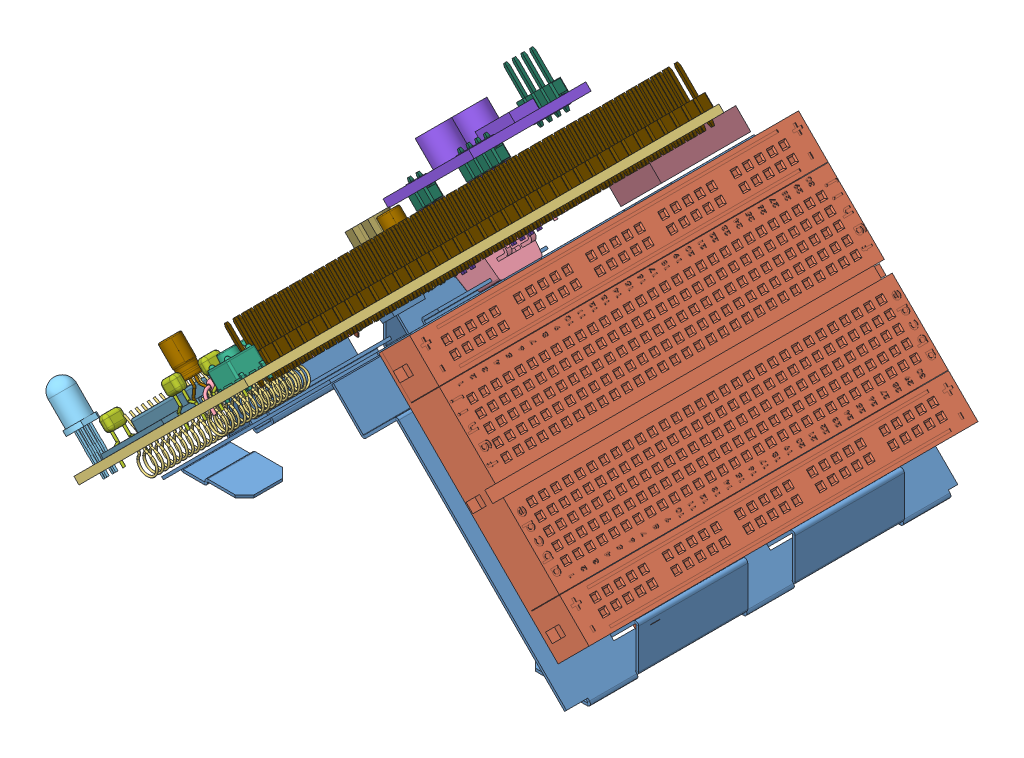
SolidWorks assembly board holder, configuration Default. Lengths in mm.
Overall size (106.21 104.29 116.2).
93 component instances, 22 part files, 18 mates.
Components (placement in the parent):
- board holder-1: board holder [Default] at (0.5717 42.6452 0.4358) x (0 0 -1) z (-0.707107 -0.707107 0) size (82.5 68.22 68.22)
- Breadboard 400-1: Breadboard 400 [Default] at (20.1582 24.8342 -10.9913) x (0 0 1) z (-0.707107 0.707107 0) size (83.85 9.2 55.35)
- MSE_duinoR5_1a-1: MSE_duinoR5_1a [Default] at (-32.0399 20.1527 23.2606) x (-0.00206 -0.00206 -0.999996) z (0.707104 0.707104 -0.002913) size (116.05 27.86 50.4)
  - flexypin-1: flexypin [Default] at (-20.41 0.2848 13.3424) x (-0.010953 -0.001001 0.99994) z (-0.000011 0.999999 0.001001) size (4.48 0.4 10.4)
  - flexypin-2: flexypin [Default] at (-19.14 0.2848 13.3424) x (-0.010953 -0.001001 0.99994) z (-0.000011 0.999999 0.001001) size (4.48 0.4 10.4)
  - flexypin-3: flexypin [Default] at (-17.87 0.2848 13.3424) x (-0.010953 -0.001001 0.99994) z (-0.000011 0.999999 0.001001) size (4.48 0.4 10.4)
  - flexypin-4: flexypin [Default] at (-16.6 0.2848 13.3424) x (-0.010953 -0.001001 0.99994) z (-0.000011 0.999999 0.001001) size (4.48 0.4 10.4)
  - flexypin-5: flexypin [Default] at (-15.33 0.2848 13.3424) x (-0.010953 -0.001001 0.99994) z (-0.000011 0.999999 0.001001) size (4.48 0.4 10.4)
  - flexypin-6: flexypin [Default] at (-14.06 0.2848 13.3424) x (-0.010953 -0.001001 0.99994) z (-0.000011 0.999999 0.001001) size (4.48 0.4 10.4)
  - flexypin-7: flexypin [Default] at (-12.79 0.2848 13.3424) x (-0.010953 -0.001001 0.99994) z (-0.000011 0.999999 0.001001) size (4.48 0.4 10.4)
  - flexypin-8: flexypin [Default] at (-11.52 0.2848 13.3424) x (-0.010953 -0.001001 0.99994) z (-0.000011 0.999999 0.001001) size (4.48 0.4 10.4)
  - flexypin-9: flexypin [Default] at (-10.25 0.2848 13.3424) x (-0.010953 -0.001001 0.99994) z (-0.000011 0.999999 0.001001) size (4.48 0.4 10.4)
  - flexypin-10: flexypin [Default] at (-8.98 0.2848 13.3424) x (-0.010953 -0.001001 0.99994) z (-0.000011 0.999999 0.001001) size (4.48 0.4 10.4)
  - flexypin-11: flexypin [Default] at (-7.71 0.2848 13.3424) x (-0.010953 -0.001001 0.99994) z (-0.000011 0.999999 0.001001) size (4.48 0.4 10.4)
  - flexypin-12: flexypin [Default] at (-6.44 0.2848 13.3424) x (-0.010953 -0.001001 0.99994) z (-0.000011 0.999999 0.001001) size (4.48 0.4 10.4)
  - flexypin-13: flexypin [Default] at (-5.17 0.2848 13.3424) x (-0.010953 -0.001001 0.99994) z (-0.000011 0.999999 0.001001) size (4.48 0.4 10.4)
  - flexypin-14: flexypin [Default] at (-3.9 0.2848 13.3424) x (-0.010953 -0.001001 0.99994) z (-0.000011 0.999999 0.001001) size (4.48 0.4 10.4)
  - flexypin-15: flexypin [Default] at (-0.8568 0.1483 9.8155) x (-0.999939 -0.001001 -0.010978) z (-0.001001 0.999999 -0.000011) size (4.48 0.4 10.4)
  - flexypin-16: flexypin [Default] at (-20.41 0.1483 -7.5876) x (-0.003303 -0.001001 0.999994) z (-0.000003 0.999999 0.001001) size (4.48 0.4 10.4)
  - flexypin-17: flexypin [Default] at (-0.8568 0.1483 8.5455) x (-0.999939 -0.001001 -0.010978) z (-0.001001 0.999999 -0.000011) size (4.48 0.4 10.4)
  - flexypin-18: flexypin [Default] at (-0.8568 0.1483 7.2755) x (-0.999939 -0.001001 -0.010978) z (-0.001001 0.999999 -0.000011) size (4.48 0.4 10.4)
  - flexypin-19: flexypin [Default] at (-0.8568 0.1483 6.0055) x (-0.999939 -0.001001 -0.010978) z (-0.001001 0.999999 -0.000011) size (4.48 0.4 10.4)
  - flexypin-20: flexypin [Default] at (-0.8568 0.1483 4.7355) x (-0.999939 -0.001001 -0.010978) z (-0.001001 0.999999 -0.000011) size (4.48 0.4 10.4)
  - flexypin-21: flexypin [Default] at (-0.8568 0.1483 3.4655) x (-0.999939 -0.001001 -0.010978) z (-0.001001 0.999999 -0.000011) size (4.48 0.4 10.4)
  - flexypin-22: flexypin [Default] at (-0.8568 0.1483 2.1955) x (-0.999939 -0.001001 -0.010978) z (-0.001001 0.999999 -0.000011) size (4.48 0.4 10.4)
  - flexypin-23: flexypin [Default] at (-0.8568 0.1483 0.9255) x (-0.999939 -0.001001 -0.010978) z (-0.001001 0.999999 -0.000011) size (4.48 0.4 10.4)
  - flexypin-24: flexypin [Default] at (-0.8568 0.1483 -0.3445) x (-0.999939 -0.001001 -0.010978) z (-0.001001 0.999999 -0.000011) size (4.48 0.4 10.4)
  - flexypin-25: flexypin [Default] at (-0.8568 0.1483 -1.6145) x (-0.999939 -0.001001 -0.010978) z (-0.001001 0.999999 -0.000011) size (4.48 0.4 10.4)
  - flexypin-26: flexypin [Default] at (-0.8568 0.1483 -2.8845) x (-0.999939 -0.001001 -0.010978) z (-0.001001 0.999999 -0.000011) size (4.48 0.4 10.4)
  - flexypin-27: flexypin [Default] at (-0.8568 0.1483 -4.1545) x (-0.999939 -0.001001 -0.010978) z (-0.001001 0.999999 -0.000011) size (4.48 0.4 10.4)
  - flexypin-28: flexypin [Default] at (-19.14 0.1483 -7.5876) x (-0.003303 -0.001001 0.999994) z (-0.000003 0.999999 0.001001) size (4.48 0.4 10.4)
  - flexypin-29: flexypin [Default] at (-17.87 0.1483 -7.5876) x (-0.003303 -0.001001 0.999994) z (-0.000003 0.999999 0.001001) size (4.48 0.4 10.4)
  - flexypin-30: flexypin [Default] at (-16.6 0.1483 -7.5876) x (-0.003303 -0.001001 0.999994) z (-0.000003 0.999999 0.001001) size (4.48 0.4 10.4)
  - flexypin-31: flexypin [Default] at (-15.33 0.1483 -7.5876) x (-0.003303 -0.001001 0.999994) z (-0.000003 0.999999 0.001001) size (4.48 0.4 10.4)
  - flexypin-32: flexypin [Default] at (-14.06 0.1483 -7.5876) x (-0.003303 -0.001001 0.999994) z (-0.000003 0.999999 0.001001) size (4.48 0.4 10.4)
  - flexypin-33: flexypin [Default] at (-12.79 0.1483 -7.5876) x (-0.003303 -0.001001 0.999994) z (-0.000003 0.999999 0.001001) size (4.48 0.4 10.4)
  - flexypin-34: flexypin [Default] at (-11.52 0.1483 -7.5876) x (-0.003303 -0.001001 0.999994) z (-0.000003 0.999999 0.001001) size (4.48 0.4 10.4)
  - flexypin-35: flexypin [Default] at (-10.25 0.1483 -7.5876) x (-0.003303 -0.001001 0.999994) z (-0.000003 0.999999 0.001001) size (4.48 0.4 10.4)
  - flexypin-36: flexypin [Default] at (-8.98 0.1483 -7.5876) x (-0.003303 -0.001001 0.999994) z (-0.000003 0.999999 0.001001) size (4.48 0.4 10.4)
  - flexypin-37: flexypin [Default] at (-7.71 0.1483 -7.5876) x (-0.003303 -0.001001 0.999994) z (-0.000003 0.999999 0.001001) size (4.48 0.4 10.4)
  - flexypin-38: flexypin [Default] at (-6.44 0.1483 -7.5876) x (-0.003303 -0.001001 0.999994) z (-0.000003 0.999999 0.001001) size (4.48 0.4 10.4)
  - flexypin-39: flexypin [Default] at (-5.17 0.1483 -7.5876) x (-0.003303 -0.001001 0.999994) z (-0.000003 0.999999 0.001001) size (4.48 0.4 10.4)
  - flexypin-40: flexypin [Default] at (-3.9 0.1483 -7.5876) x (-0.003303 -0.001001 0.999994) z (-0.000003 0.999999 0.001001) size (4.48 0.4 10.4)
  - 4k7 Resistor-2: 4k7 Resistor [Default] at (53.3526 1.6846 -2.2179) x (1 -0.000227 0) z (0 0 1) size (10.63 5.13 2.14)
  - 4k7 Resistor-3: 4k7 Resistor [Default] at (53.4006 1.1919 4.1961) x (1 -0.000227 0) z (0 0 1) size (10.63 5.13 2.14)
  - 4k7 Resistor-4: 4k7 Resistor [Default] at (53.3476 1.5334 20.6721) x (1 -0.000227 0) z (0 0 1) size (10.63 5.13 2.14)
  - 4k7 Resistor-5: 4k7 Resistor [Default] at (40.5664 1.561 -1.0614) x (1 -0.000286 0) z (0 0 1) size (10.63 5.13 2.14)
  - 4k7 Resistor-6: 4k7 Resistor [Default] at (17.8933 1.5357 -12.7339) x (-1 -0.000286 0) z (0 0 -1) size (10.63 5.13 2.14)
  - 4k7 Resistor-8: 4k7 Resistor [Default] at (53.4026 1.5613 0.9311) x (1 -0.000227 0) z (0 0 1) size (10.63 5.13 2.14)
  - APA-106-F8-1: APA-106-F8 [Default] at (-24.7776 1.0639 -10.8804) x (1 0 0) z (0 1 0) size (5.8 5.34 16.88)
  - B3F-10XX-1: B3F-10XX [Default] at (-24.9981 -0.2 31.2137) x (0.011028 0 0.999939) z (0 1 0) size (6.85 6 7)
  - B3F-10XX-2: B3F-10XX [Default] at (8.2644 -0.2 -9.7242) x (-0.011162 0 -0.999938) z (0 1 0) size (6.85 6 7)
  - C050024X044_C050024X044-1: C050024X044_C050024X044 [Default] at (13.928 -2.6 11.4866) x (0 0 -1) z (0 1 0) size (5.59 2.2 8.4)
  - C050024X044_C050024X044-2: C050024X044_C050024X044 [Default] at (23.427 -2.6 11.5366) x (0 0 -1) z (0 1 0) size (5.59 2.2 8.4)
  - C050024X044_C050024X044-3: C050024X044_C050024X044 [Default] at (-26.23 -2.6 16.8966) x (0 0 -1) z (0 1 0) size (5.59 2.2 8.4)
  - C050024X044_C050024X044-4: C050024X044_C050024X044 [Default] at (62.1347 -2.5253 11.5231) x (0 0 -1) z (0 1 0) size (5.59 2.2 8.4)
  - dual motor controller-1: dual motor controller [Default] at (49.5705 11.1526 10.8742) x (0.010236 0 0.999948) z (-0.999948 0 0.010236) size (25.07 7.1 24.93)
  - Electrolitic Capacitor Radial 4x7-1: Electrolitic Capacitor Radial 4x7 [Default] at (27.11 3.9479 11.826) x (0 0 1) z (-1 0 0) size (5.5 11.95 4)
  - Electrolitic Capacitor Radial 4x7-2: Electrolitic Capacitor Radial 4x7 [Default] at (-22.5429 3.9479 16.8049) x (0.001608 0 0.999999) z (-0.999999 0 0.001608) size (5.5 11.95 4)
  - 4k7 Resistor-16: 4k7 Resistor [Default] at (-20.9402 1.4587 21.7985) x (1 -0.000227 -0.00002) z (0.00002 0 1) size (10.63 5.13 2.14)
  - C050024X044_C050024X044-5: C050024X044_C050024X044 [Default] at (-24.477 -2.6 25.6336) x (1 0 0) z (0 1 0) size (5.59 2.2 8.4)
  - LED3MM red-1: LED3MM red [Default] at (9.356 1.075 -2.6592) x (0 0 -1) z (0 1 0) size (3.05 3.04 9.56)
  - C050024X044_C050024X044-6: C050024X044_C050024X044 [Default] at (-18.534 -2.6 -12.0344) x (1 0 0) z (0 1 0) size (5.59 2.2 8.4)
  - Spike_PT10_Trimmer-1: Spike_PT10_Trimmer [Varsayılan] at (30.259 1.5 -8.2244) x (0 0 -1) z (1 0 0) size (11.45 11 11.45)
  - TO-92 formed-1: TO-92 formed [Default] at (28.939 6.2 -0.5284) size (5.78 13.88 3.3)
  - TO-92 formed-2: TO-92 formed [Default] at (29.015 6.2 4.0436) size (5.78 13.88 3.3)
  - USB_AP_PWR-1: USB_AP_PWR [Default] at (67.776 -1.3 10.1914) x (1 0 0) z (0 -1 0) size (20.64 12.02 7.83)
  - ESP32-S3-WROOM-1: ESP32-S3-WROOM [Default] at (-15.0428 0 2.7484) x (0 0 -1) z (1 0 0) size (18.02 3.16 25.51)
  - Header 2_54 Vertical 1x2-3: Header 2_54 Vertical 1x2 [Default] at (70.468 1.25 -12.1104) x (1 0 0) z (0 1 0) size (5.08 2.5 11)
  - Header 2_54 Vertical 1x2-4: Header 2_54 Vertical 1x2 [Default] at (57.679 14.0026 14.1063) x (-0.010236 0 -0.999948) z (0 1 0) size (5.08 2.5 11)
  - Header 2_54 Vertical 1x2-5: Header 2_54 Vertical 1x2 [Default] at (57.731 14.0026 19.1861) x (-0.010236 0 -0.999948) z (0 1 0) size (5.08 2.5 11)
  - Dip SW 4-1: Dip SW 4 [Default] at (52.7107 0.05 -8.7189) x (1 0 0) z (0 1 0) size (12.14 8.28 7.35)
  - JP2N_Recept-1: JP2N_Recept [Default] at (42.2934 0 17.644) x (0 0 -1) z (0 1 0) size (4.68 2.52 11.5)
  - JP2N_Recept-2: JP2N_Recept [Default] at (42.2934 0 12.564) x (0 0 -1) z (0 1 0) size (4.68 2.52 11.5)
  - JP2N_Recept-3: JP2N_Recept [Default] at (38.0836 0 3.6768) x (-0.010236 0 -0.999948) z (0 1 0) size (4.68 2.52 11.5)
  - Header 2_54 Vertical 1x37-2: Header 2_54 Vertical 1x37 [Default] at (70.849 1.25 31.0696) x (1 0 0) z (0 1 0) size (93.98 2.5 11)
  - Header 2_54 Vertical 1x37-3: Header 2_54 Vertical 1x37 [Default] at (70.849 1.25 28.5296) x (1 0 0) z (0 1 0) size (93.98 2.5 11)
  - Header 2_54 Vertical 1x37-4: Header 2_54 Vertical 1x37 [Default] at (70.849 1.25 33.6096) x (1 0 0) z (0 1 0) size (93.98 2.5 11)
  - Header 2_54 Vertical 1x2-6: Header 2_54 Vertical 1x2 [Default] at (42.4398 9.9026 14.2623) x (-0.010236 0 -0.999948) z (0 -1 0) size (5.08 2.5 11)
  - Header 2_54 Vertical 1x2-7: Header 2_54 Vertical 1x2 [Default] at (38.159 9.9026 5.4157) x (-0.010236 0 -0.999948) z (0 -1 0) size (5.08 2.5 11)
  - Header 2_54 Vertical 1x2-8: Header 2_54 Vertical 1x2 [Default] at (42.4918 9.9026 19.3421) x (-0.010236 0 -0.999948) z (0 -1 0) size (5.08 2.5 11)
  - SP1117-1: SP1117 [Default] at (18.3683 -1.4981 14.8788) x (-1 0 0) z (0 -1 0) size (6.7 6.67 1.8)
  - USB_C CU32-16-1: USB_C CU32-16 [Default] at (72.474 1.58 -3.0074) x (0 0 -1) z (1 0 0) size (8.94 4.8 9.1)
  - pcb r5.1-1: pcb r5.1 [Default] at (-29.4833 -1.5253 36.1611) size (100.42 1.5 50.4)
  - 4k7 Resistor-17: 4k7 Resistor [Default] at (53.3476 1.5334 17.4221) x (1 -0.000227 0) z (0 0 1) size (10.63 5.13 2.14)
  - 4k7 Resistor-18: 4k7 Resistor [Default] at (53.3476 1.5334 14.1721) x (1 -0.000227 0) z (0 0 1) size (10.63 5.13 2.14)
  - 4k7 Resistor-19: 4k7 Resistor [Default] at (53.3476 1.5334 10.9221) x (1 -0.000227 0) z (0 0 1) size (10.63 5.13 2.14)
  - 4k7 Resistor-20: 4k7 Resistor [Default] at (53.3476 1.5334 7.6721) x (1 -0.000227 0) z (0 0 1) size (10.63 5.13 2.14)
  - 4k7 Resistor-21: 4k7 Resistor [Default] at (40.5664 1.561 2.6886) x (1 -0.000286 0) z (0 0 1) size (10.63 5.13 2.14)
  - 4k7 Resistor-22: 4k7 Resistor [Default] at (17.8933 1.5357 -9.7339) x (-1 -0.000286 0) z (0 0 -1) size (10.63 5.13 2.14)
  - 4k7 Resistor-23: 4k7 Resistor [Default] at (17.8933 1.5357 -6.5339) x (-1 -0.000286 0) z (0 0 -1) size (10.63 5.13 2.14)
  - 4k7 Resistor-24: 4k7 Resistor [Default] at (17.8933 1.5357 -3.3339) x (-1 -0.000286 0) z (0 0 -1) size (10.63 5.13 2.14)
  - D2PAK-2-1: D2PAK-2 [Default] at (53.5908 -1.5253 -7.6299) x (-1 0 0) z (0 -1 0) size (10 15.62 5.08)
Mates (geometry in assembly coordinates):
- Coincident55: coincident: plane of board holder-1 through (-6.8883 35.963 14.9796) normal (0 0 -1); plane of upperBrdHolder-3 through (0.0656 35.5969 14.9796) normal (0 0 1)
- Coincident56: coincident anti-aligned: plane of board holder-1 through (0.1828 43.0341 0.4358) normal (-0.707107 0.707107 0); plane of upperBrdHolder-3 through (-13.9719 28.8794 14.9796) normal (0.707107 -0.707107 0)
- Coincident57: coincident: plane of board holder-1 through (-1.6062 41.2451 14.6796) normal (-0.707107 -0.707107 0); plane of upperBrdHolder-3 through (0.0656 35.5969 14.4296) normal (0 0 -1)
- Coincident58: coincident anti-aligned: plane of upperBrdHolder-3 through (0.0656 35.5969 14.4296) normal (0 0 -1); plane of upperBrdHolder-4 through (0.8027 35.5969 14.4296) normal (0 0 1)
- Coincident59: coincident anti-aligned: plane of board holder-1 through (0.6855 43.0341 0.4358) normal (0.707107 0.707107 0); plane of upperBrdHolder-4 through (14.8402 28.8794 13.8796) normal (-0.707107 -0.707107 0)
- Coincident60: coincident: plane of board holder-1 through (2.4745 41.2451 14.1796) normal (0.707107 -0.707107 0); plane of upperBrdHolder-4 through (0.8027 35.5969 14.4296) normal (0 0 1)
- Parallel8: parallel aligned: plane of board holder-1 through (-42.2436 0.6077 32.9358) normal (0 0 1); plane of lowerBrdHoler-4 through (3.7871 14.3107 17.3858) normal (0 0 1)
- Coincident69: coincident anti-aligned: plane of board holder-1 through (-27.96 14.8913 17.3858) normal (0 0 -1); plane of lowerBrdHoler-4 through (3.7871 14.3107 17.3858) normal (0 0 1)
- Coincident70: coincident anti-aligned: plane of board holder-1 through (0.1828 43.0341 0.4358) normal (-0.707107 0.707107 0); plane of lowerBrdHoler-4 through (-28.5406 14.3107 17.3858) normal (0.707107 -0.707107 0)
- Coincident71: coincident anti-aligned: plane of board holder-1 through (-24.9658 17.8854 22.6266) normal (-0.707107 -0.707107 0); plane of lowerBrdHoler-4 through (-8.802 1.7216 35.3504) normal (0.707107 0.707107 0)
- Coincident72: coincident anti-aligned: plane of board holder-1 through (0.6855 43.0341 0.4358) normal (0.707107 0.707107 0); plane of lowerBBrdHoler-3 through (41.0762 2.6434 16.2858) normal (-0.707107 -0.707107 0)
- Coincident74: coincident anti-aligned: plane of lowerBBrdHoler-3 through (-2.9188 14.3107 16.8358) normal (0 0 1); plane of lowerBrdHoler-4 through (3.7871 14.3107 16.8358) normal (0 0 -1)
- Coincident75: coincident aligned: plane of lowerBBrdHoler-3 through (-2.9188 14.3107 16.2858) normal (0 1 0); plane of lowerBrdHoler-4 through (3.7871 14.3107 17.3858) normal (0 1 0)
- Coincident76: coincident anti-aligned: plane of board holder-1 through (0.6855 43.0341 0.4358) normal (0.707107 0.707107 0); plane of Breadboard 400-1 through (19.5218 24.1978 -10.9913) normal (-0.707107 -0.707107 0)
- Coincident77: coincident anti-aligned: plane of board holder-1 through (38.3063 5.152 0.4358) normal (-0.707107 0.707107 0); plane of Breadboard 400-1 through (38.4369 5.2827 -51.9913) normal (0.707107 -0.707107 0)
- Parallel9: parallel anti-aligned: plane of board holder-1 through (0.1828 43.0341 0.4358) normal (-0.707107 0.707107 0); plane of MSE_duinoR5_1a-1/pcb r5.1-1 through (-5.3309 44.7046 52.6384) normal (0.707107 -0.707107 0)
- Concentric1: concentric aligned: cylinder of board holder-1 through (-19.1495 23.7018 -11.6542) axis (0.707107 -0.707107 0) radius 1.5; cylinder of MSE_duinoR5_1a-1/pcb r5.1-1 through (-23.8022 28.3546 -11.6542) axis (0.707107 -0.707107 0) radius 1.4
- Coincident79: coincident anti-aligned: plane of board holder-1 through (0.1828 43.0341 0.4358) normal (-0.707107 0.707107 0); plane of MSE_duinoR5_1a-1/D2PAK-2-1 through (-32.8747 9.9765 -30.3077) normal (0.707107 -0.707107 0)
